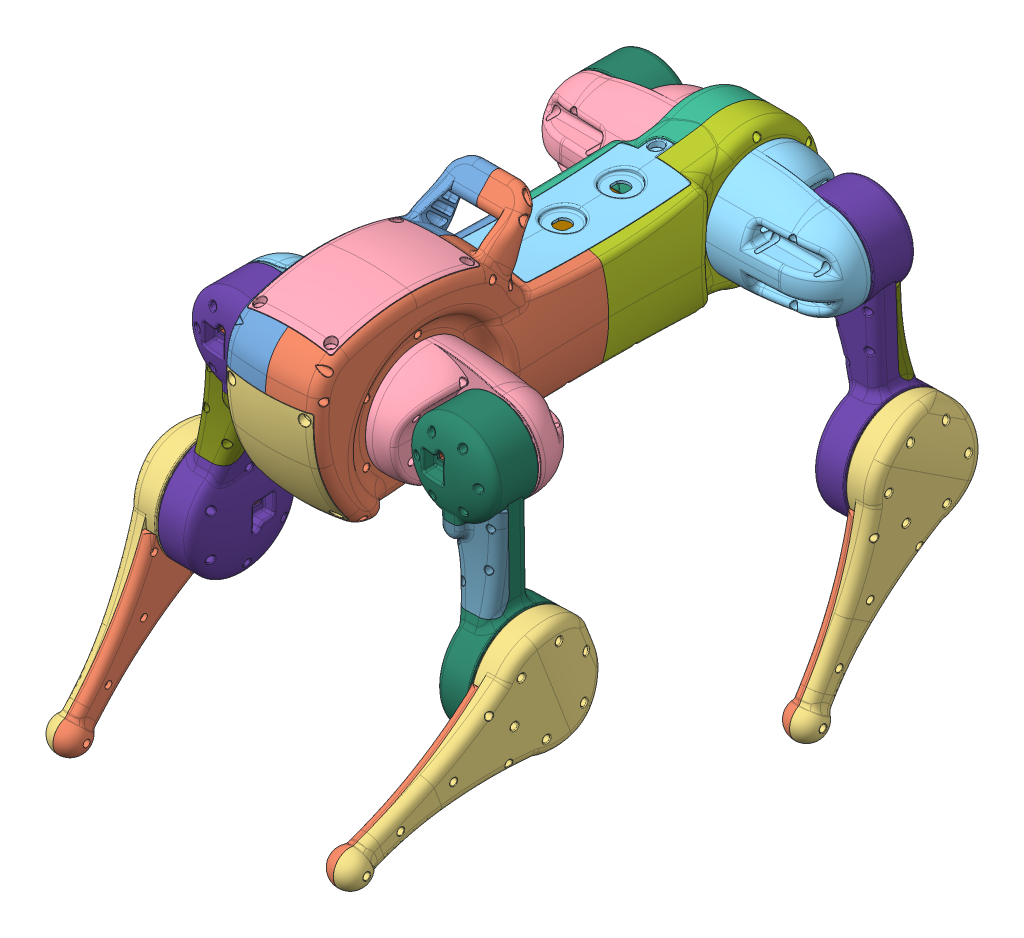
SolidWorks assembly ROBOT DOG, configuration Default. Lengths in mm.
Overall size (409.03 517.61 692.63).
101 component instances, 23 part files, 143 mates.
Components (placement in the parent):
- RIGHT FRONT TORSO - ROBOT DOG-1: RIGHT FRONT TORSO - ROBOT DOG [Default] at origin size (84.53 210.28 299.93)
- MirrorLEFT FRONT TORSO - ROBOT DOG-3: MirrorLEFT FRONT TORSO - ROBOT DOG [Default] x (-1 0 0) z (0 0 -1) size (91.07 210.28 299.93)
- COVER OF THE CAMERA BOARD - ROBOT DOG-1: COVER OF THE CAMERA BOARD - ROBOT DOG [Default] at origin size (89.79 121.01 49.11)
- COVER OF THE COMPUTER BOARD - ROBOT DOG-1: COVER OF THE COMPUTER BOARD - ROBOT DOG [Default] at origin size (87.15 28.45 157.74)
- COVER OF THE BATTERY - ROBOT DOG-1: COVER OF THE BATTERY - ROBOT DOG [Default] at origin size (83.94 31.1 211.37)
- RIGHT BACK TORSO - ROBOT DOG-2: RIGHT BACK TORSO - ROBOT DOG [Default] at origin size (84.66 140 246.51)
- MirrorLEFT BACK TORSO - ROBOT DOG-6: MirrorLEFT BACK TORSO - ROBOT DOG [Default] x (-1 0 0) z (0 0 -1) size (91.16 140 246.51)
- CONTROLLER BEHIND OF THE BATTERY - ROBOT DOG 38MM WITDH-1: CONTROLLER BEHIND OF THE BATTERY - ROBOT DOG 38MM WITDH [Default] at (0 -15.25 0) x (1 0 0) z (0 1 0) size (50 140 21.9)
- BATTERY - ROBOT DOG-1: BATTERY - ROBOT DOG [Default] at (0 8.05 -7) x (1 0 0) z (0 1 0) size (69 169 39)
- BIG PART - MOTOR 6-1: BIG PART - MOTOR 6 [Default] at (-113 -0.0192 -188.18) x (0 0.001455 0.999999) z (0.048855 0.998805 -0.001453) size (39.01 74 74)
  - PART 2 - MOTOR 6 - ROBOT DOG-1: PART 2 - MOTOR 6 - ROBOT DOG [Default] at origin size (33.16 74 74)
  - BIGGER CONTROLLER - ROBOT DOG-1: BIGGER CONTROLLER - ROBOT DOG [Default] at (-15.88 0 0) x (0 -1 0) z (0 0 -1) size (45 7.4 45)
- BIG PART - MOTOR 6-2: BIG PART - MOTOR 6 [Default] at (-113 0.0018 188.18) x (0 -0.000135 -1) z (0.008141 0.999967 -0.000135) size (39.01 74 74)
  - PART 2 - MOTOR 6 - ROBOT DOG-1: PART 2 - MOTOR 6 - ROBOT DOG [Default] at origin size (33.16 74 74)
  - BIGGER CONTROLLER - ROBOT DOG-1: BIGGER CONTROLLER - ROBOT DOG [Default] at (-15.88 0 0) x (0 -1 0) z (0 0 -1) size (45 7.4 45)
- BIG PART - MOTOR 6-3: BIG PART - MOTOR 6 [Default] at (113 0.1463 -188.1792) x (0 -0.011103 0.999938) z (-0.026827 0.999578 0.011099) size (39.01 74 74)
  - PART 2 - MOTOR 6 - ROBOT DOG-1: PART 2 - MOTOR 6 - ROBOT DOG [Default] at origin size (33.16 74 74)
  - BIGGER CONTROLLER - ROBOT DOG-1: BIGGER CONTROLLER - ROBOT DOG [Default] at (-15.88 0 0) x (0 -1 0) z (0 0 -1) size (45 7.4 45)
- BIG PART - MOTOR 6-4: BIG PART - MOTOR 6 [Default] at (113 0.1616 188.179) x (0 -0.012263 -0.999925) z (-0.027212 0.999555 -0.012259) size (39.01 74 74)
  - PART 2 - MOTOR 6 - ROBOT DOG-1: PART 2 - MOTOR 6 - ROBOT DOG [Default] at origin size (33.16 74 74)
  - BIGGER CONTROLLER - ROBOT DOG-1: BIGGER CONTROLLER - ROBOT DOG [Default] at (-15.88 0 0) x (0 -1 0) z (0 0 -1) size (45 7.4 45)
- SMALL PART - MOTOR 6-1: SMALL PART - MOTOR 6 [Default] at (113 -0.0619 169.9504) x (0 -0.012263 -0.999925) z (0.5 -0.86596 0.01062) size (5.8 74 74)
  - PART 1 - MOTOR 6 - ROBOT DOG-2: PART 1 - MOTOR 6 - ROBOT DOG [Default] at origin size (4.8 74 74)
  - SMALL CONTROLLER - ROBOT DOG-1: SMALL CONTROLLER - ROBOT DOG [Default] at (1.9 0 0) x (1 0 0) z (0 -0.5 0.866025) size (1 40.5 45)
- SMALL PART - MOTOR 6-2: SMALL PART - MOTOR 6 [Default] at (113 -0.0561 -169.9503) x (0 -0.011103 0.999938) z (0.5 0.865972 0.009616) size (5.8 74 74)
  - PART 1 - MOTOR 6 - ROBOT DOG-2: PART 1 - MOTOR 6 - ROBOT DOG [Default] at origin size (4.8 74 74)
  - SMALL CONTROLLER - ROBOT DOG-1: SMALL CONTROLLER - ROBOT DOG [Default] at (1.9 0 0) x (1 0 0) z (0 -0.5 0.866025) size (1 40.5 45)
- SMALL PART - MOTOR 6-3: SMALL PART - MOTOR 6 [Default] at (-113 0.0073 -169.95) x (0 0.001455 0.999999) z (-0.5 -0.866024 0.00126) size (5.8 74 74)
  - PART 1 - MOTOR 6 - ROBOT DOG-2: PART 1 - MOTOR 6 - ROBOT DOG [Default] at origin size (4.8 74 74)
  - SMALL CONTROLLER - ROBOT DOG-1: SMALL CONTROLLER - ROBOT DOG [Default] at (1.9 0 0) x (1 0 0) z (0 -0.5 0.866025) size (1 40.5 45)
- SMALL PART - MOTOR 6-4: SMALL PART - MOTOR 6 [Default] at (-113 -0.0007 169.95) x (0 -0.000135 -1) z (-0.5 0.866025 -0.000117) size (5.8 74 74)
  - PART 1 - MOTOR 6 - ROBOT DOG-2: PART 1 - MOTOR 6 - ROBOT DOG [Default] at origin size (4.8 74 74)
  - SMALL CONTROLLER - ROBOT DOG-1: SMALL CONTROLLER - ROBOT DOG [Default] at (1.9 0 0) x (1 0 0) z (0 -0.5 0.866025) size (1 40.5 45)
- COVER OF THE THIGN - ROBOT DOG-1: COVER OF THE THIGN - ROBOT DOG [Default] at (113 0.2046 191.6787) x (0.99963 0.02721 -0.000334) z (0 0.012263 0.999925) size (62.68 88.46 26.31)
- COVER OF THE THIGN - ROBOT DOG-2: COVER OF THE THIGN - ROBOT DOG [Default] at (-113 -0.0243 -191.68) x (-0.998806 0.048855 -0.000071) z (0 -0.001455 -0.999999) size (62.68 88.46 26.31)
- THIGN - ROBOT DOG-1: THIGN - ROBOT DOG [Default] at (-113 -0.0243 -191.68) x (-0.998806 0.048855 -0.000071) z (0 -0.001455 -0.999999) size (90.79 271.35 112.7)
- THIGN - ROBOT DOG-2: THIGN - ROBOT DOG [Default] at (113 0.2046 191.6787) x (0.99963 0.02721 -0.000334) z (0 0.012263 0.999925) size (90.79 271.35 112.7)
- MirrorCOVER OF THE THIGN - ROBOT DOG-4: MirrorCOVER OF THE THIGN - ROBOT DOG [Default] at (-113 0.0022 191.68) x (-0.999967 0.008141 -0.000001) z (0 -0.000135 -1) size (62.68 88.46 26.31)
- MirrorCOVER OF THE THIGN - ROBOT DOG-5: MirrorCOVER OF THE THIGN - ROBOT DOG [Default] at (113 0.1852 -191.679) x (0.99964 0.026825 0.000298) z (0 -0.011103 0.999938) size (62.68 88.46 26.31)
- MirrorANOTHER THIGN - ROBOT DOG-3: MirrorANOTHER THIGN - ROBOT DOG [Default] at (113 0.1852 -191.679) x (0.99964 0.026825 0.000298) z (0 -0.011103 0.999938) size (90.79 271.35 112.7)
- MirrorANOTHER THIGN - ROBOT DOG-4: MirrorANOTHER THIGN - ROBOT DOG [Default] at (-113 0.0022 191.68) x (-0.999967 0.008141 -0.000001) z (0 -0.000135 -1) size (90.79 271.35 112.7)
- BIG PART MOTOR 8-1: BIG PART MOTOR 8 [Default] at (24.425 0 175) size (30.55 96.7 96.7)
  - PART 2 - MOTOR 8 - ROBOT DOG-1: PART 2 - MOTOR 8 - ROBOT DOG [Default] at origin size (24.65 96.7 96.7)
  - BIGGER CONTROLLER - ROBOT DOG-1: BIGGER CONTROLLER - ROBOT DOG [Default] at (-11.675 0 0) x (0 0 1) z (0 -1 0) size (45 7.4 45)
- SMALL PART MOTOR 8-1: SMALL PART MOTOR 8 [Default] at (39.725 0 175) x (1 0 0) z (0 -0.859829 0.510583) size (8.45 96.7 96.7)
  - PART 1 - MOTOR 8 - ROBOT DOG-1: PART 1 - MOTOR 8 - ROBOT DOG [Default] at origin size (7.45 96.7 96.7)
  - SMALL CONTROLLER - ROBOT DOG-1: SMALL CONTROLLER - ROBOT DOG [Default] at (3.225 0 0) x (1 0 0) z (0 -0.5 0.866025) size (1 40.5 45)
- BIG PART MOTOR 8-2: BIG PART MOTOR 8 [Default] at (24.425 0 -175) size (30.55 96.7 96.7)
  - PART 2 - MOTOR 8 - ROBOT DOG-1: PART 2 - MOTOR 8 - ROBOT DOG [Default] at origin size (24.65 96.7 96.7)
  - BIGGER CONTROLLER - ROBOT DOG-1: BIGGER CONTROLLER - ROBOT DOG [Default] at (-11.675 0 0) x (0 0 1) z (0 -1 0) size (45 7.4 45)
- BIG PART MOTOR 8-3: BIG PART MOTOR 8 [Default] at (-24.425 0 175) x (-1 0 0) z (0 0 -1) size (30.55 96.7 96.7)
  - PART 2 - MOTOR 8 - ROBOT DOG-1: PART 2 - MOTOR 8 - ROBOT DOG [Default] at origin size (24.65 96.7 96.7)
  - BIGGER CONTROLLER - ROBOT DOG-1: BIGGER CONTROLLER - ROBOT DOG [Default] at (-11.675 0 0) x (0 0 1) z (0 -1 0) size (45 7.4 45)
- BIG PART MOTOR 8-4: BIG PART MOTOR 8 [Default] at (-24.425 0 -175) x (-1 0 0) z (0 0 -1) size (30.55 96.7 96.7)
  - PART 2 - MOTOR 8 - ROBOT DOG-1: PART 2 - MOTOR 8 - ROBOT DOG [Default] at origin size (24.65 96.7 96.7)
  - BIGGER CONTROLLER - ROBOT DOG-1: BIGGER CONTROLLER - ROBOT DOG [Default] at (-11.675 0 0) x (0 0 1) z (0 -1 0) size (45 7.4 45)
- SMALL PART MOTOR 8-2: SMALL PART MOTOR 8 [Default] at (39.725 0 -175) x (1 0 0) z (0 0.871524 -0.490354) size (8.45 96.7 96.7)
  - PART 1 - MOTOR 8 - ROBOT DOG-1: PART 1 - MOTOR 8 - ROBOT DOG [Default] at origin size (7.45 96.7 96.7)
  - SMALL CONTROLLER - ROBOT DOG-1: SMALL CONTROLLER - ROBOT DOG [Default] at (3.225 0 0) x (1 0 0) z (0 -0.5 0.866025) size (1 40.5 45)
- SMALL PART MOTOR 8-3: SMALL PART MOTOR 8 [Default] at (-39.725 0 175) x (-1 0 0) z (0 0.866093 0.499883) size (8.45 96.7 96.7)
  - PART 1 - MOTOR 8 - ROBOT DOG-1: PART 1 - MOTOR 8 - ROBOT DOG [Default] at origin size (7.45 96.7 96.7)
  - SMALL CONTROLLER - ROBOT DOG-1: SMALL CONTROLLER - ROBOT DOG [Default] at (3.225 0 0) x (1 0 0) z (0 -0.5 0.866025) size (1 40.5 45)
- SMALL PART MOTOR 8-4: SMALL PART MOTOR 8 [Default] at (-39.725 0 -175) x (-1 0 0) z (0 -0.866752 -0.49874) size (8.45 96.7 96.7)
  - PART 1 - MOTOR 8 - ROBOT DOG-1: PART 1 - MOTOR 8 - ROBOT DOG [Default] at origin size (7.45 96.7 96.7)
  - SMALL CONTROLLER - ROBOT DOG-1: SMALL CONTROLLER - ROBOT DOG [Default] at (3.225 0 0) x (1 0 0) z (0 -0.5 0.866025) size (1 40.5 45)
- BIG PART MOTOR 8-5: BIG PART MOTOR 8 [Default] at (150.9736 -168.8465 -193.5559) x (0.99964 0.026825 0.000298) z (0 0.011103 -0.999938) size (30.55 96.7 96.7)
  - PART 2 - MOTOR 8 - ROBOT DOG-1: PART 2 - MOTOR 8 - ROBOT DOG [Default] at origin size (24.65 96.7 96.7)
  - BIGGER CONTROLLER - ROBOT DOG-1: BIGGER CONTROLLER - ROBOT DOG [Default] at (-11.675 0 0) x (0 0 1) z (0 -1 0) size (45 7.4 45)
- BIG PART MOTOR 8-6: BIG PART MOTOR 8 [Default] at (151.0387 -168.8102 193.7516) x (0.99963 0.02721 -0.000334) z (0 -0.012263 -0.999925) size (30.55 96.7 96.7)
  - PART 2 - MOTOR 8 - ROBOT DOG-1: PART 2 - MOTOR 8 - ROBOT DOG [Default] at origin size (24.65 96.7 96.7)
  - BIGGER CONTROLLER - ROBOT DOG-1: BIGGER CONTROLLER - ROBOT DOG [Default] at (-11.675 0 0) x (0 0 1) z (0 -1 0) size (45 7.4 45)
- BIG PART MOTOR 8-7: BIG PART MOTOR 8 [Default] at (-154.6904 -168.1881 -191.4353) x (-0.998806 0.048855 -0.000071) z (0 0.001455 0.999999) size (30.55 96.7 96.7)
  - PART 2 - MOTOR 8 - ROBOT DOG-1: PART 2 - MOTOR 8 - ROBOT DOG [Default] at origin size (24.65 96.7 96.7)
  - BIGGER CONTROLLER - ROBOT DOG-1: BIGGER CONTROLLER - ROBOT DOG [Default] at (-11.675 0 0) x (0 0 1) z (0 -1 0) size (45 7.4 45)
- BIG PART MOTOR 8-8: BIG PART MOTOR 8 [Default] at (-147.8078 -169.72 191.7028) x (-0.999967 0.008141 -0.000001) z (0 0.000135 1) size (30.55 96.7 96.7)
  - PART 2 - MOTOR 8 - ROBOT DOG-1: PART 2 - MOTOR 8 - ROBOT DOG [Default] at origin size (24.65 96.7 96.7)
  - BIGGER CONTROLLER - ROBOT DOG-1: BIGGER CONTROLLER - ROBOT DOG [Default] at (-11.675 0 0) x (0 0 1) z (0 -1 0) size (45 7.4 45)
- SMALL PART MOTOR 8-5: SMALL PART MOTOR 8 [Default] at (166.2681 -168.4361 -193.5513) x (0.99964 0.026825 0.000298) z (-0.026771 0.998201 -0.05365) size (8.45 96.7 96.7)
  - PART 1 - MOTOR 8 - ROBOT DOG-1: PART 1 - MOTOR 8 - ROBOT DOG [Default] at origin size (7.45 96.7 96.7)
  - SMALL CONTROLLER - ROBOT DOG-1: SMALL CONTROLLER - ROBOT DOG [Default] at (3.225 0 0) x (1 0 0) z (0 -0.5 0.866025) size (1 40.5 45)
- SMALL PART MOTOR 8-6: SMALL PART MOTOR 8 [Default] at (166.3331 -168.3939 193.7465) x (0.99963 0.02721 -0.000334) z (-0.025425 0.938287 0.344921) size (8.45 96.7 96.7)
  - PART 1 - MOTOR 8 - ROBOT DOG-1: PART 1 - MOTOR 8 - ROBOT DOG [Default] at origin size (7.45 96.7 96.7)
  - SMALL CONTROLLER - ROBOT DOG-1: SMALL CONTROLLER - ROBOT DOG [Default] at (3.225 0 0) x (1 0 0) z (0 -0.5 0.866025) size (1 40.5 45)
- SMALL PART MOTOR 8-7: SMALL PART MOTOR 8 [Default] at (-169.9721 -167.4406 -191.4364) x (-0.998806 0.048855 -0.000071) z (-0.013599 -0.279414 -0.960074) size (8.45 96.7 96.7)
  - PART 1 - MOTOR 8 - ROBOT DOG-1: PART 1 - MOTOR 8 - ROBOT DOG [Default] at origin size (7.45 96.7 96.7)
  - SMALL CONTROLLER - ROBOT DOG-1: SMALL CONTROLLER - ROBOT DOG [Default] at (3.225 0 0) x (1 0 0) z (0 -0.5 0.866025) size (1 40.5 45)
- SMALL PART MOTOR 8-8: SMALL PART MOTOR 8 [Default] at (-163.1073 -169.5955 191.7028) x (-0.999967 0.008141 -0.000001) z (-0.00269 -0.330238 0.943894) size (8.45 96.7 96.7)
  - PART 1 - MOTOR 8 - ROBOT DOG-1: PART 1 - MOTOR 8 - ROBOT DOG [Default] at origin size (7.45 96.7 96.7)
  - SMALL CONTROLLER - ROBOT DOG-1: SMALL CONTROLLER - ROBOT DOG [Default] at (3.225 0 0) x (1 0 0) z (0 -0.5 0.866025) size (1 40.5 45)
- COVER OF THE LEG - ROBOT DOG-1: COVER OF THE LEG - ROBOT DOG [Default] at (164.6087 -168.4408 193.747) x (-0.99963 -0.02721 0.000334) z (0.025425 -0.938287 -0.344921) size (18.15 177.43 78.27)
- COVER OF THE LEG - ROBOT DOG-2: COVER OF THE LEG - ROBOT DOG [Default] at (164.5437 -168.4823 -193.5518) x (-0.99964 -0.026825 -0.000298) z (0.014889 -0.545539 -0.837953) size (18.15 177.43 78.27)
- COVER OF THE LEG - ROBOT DOG-3: COVER OF THE LEG - ROBOT DOG [Default] at (-161.3824 -169.6095 191.7028) x (0.999967 -0.008141 0.000001) z (0.00531 0.65229 0.757951) size (18.15 177.43 78.27)
- COVER OF THE LEG - ROBOT DOG-4: COVER OF THE LEG - ROBOT DOG [Default] at (-168.2492 -167.5249 -191.4363) x (0.998806 -0.048855 0.000071) z (0.047437 0.970162 0.237771) size (18.15 177.43 78.27)
- LEG - ROBOT DOG-1: LEG - ROBOT DOG [Default] at (-168.2492 -167.5249 -191.4363) x (0.998806 -0.048855 0.000071) z (0.047437 0.970162 0.237771) size (32.62 277.86 112.7)
- LEG - ROBOT DOG-2: LEG - ROBOT DOG [Default] at (-161.3824 -169.6095 191.7028) x (0.999967 -0.008141 0.000001) z (0.00531 0.65229 0.757951) size (32.62 277.86 112.7)
- LEG - ROBOT DOG-3: LEG - ROBOT DOG [Default] at (164.6087 -168.4408 193.747) x (-0.99963 -0.02721 0.000334) z (0.025425 -0.938287 -0.344921) size (32.62 277.86 112.7)
- LEG - ROBOT DOG-4: LEG - ROBOT DOG [Default] at (164.5437 -168.4823 -193.5518) x (-0.99964 -0.026825 -0.000298) z (0.014889 -0.545539 -0.837953) size (32.62 277.86 112.7)
- SHOULDER-1: SHOULDER [Default] at (38 0 175) x (1 0 0) z (0 0.012263 0.999925) size (122.68 117.46 115.67)
- SHOULDER-2: SHOULDER [Default] at (-38 0 -175) x (-1 0 0) z (0 -0.001455 -0.999999) size (122.68 117.46 115.67)
- MirrorSHOULDER-4: MirrorSHOULDER [Default] at (-38 0 175) x (-1 0 0) z (0 -0.000135 -1) size (122.68 117.46 115.67)
- MirrorSHOULDER-5: MirrorSHOULDER [Default] at (38 0 -175) x (1 0 0) z (0 -0.011103 0.999938) size (122.68 117.46 115.67)
Mates (geometry in assembly coordinates):
- Coincident1: coincident aligned: plane of RIGHT FRONT TORSO - ROBOT DOG-1 through (0 0 0) normal (0 0 1); plane of assembly through (0 0 0) normal (0 0 1)
- Coincident2: coincident aligned: plane of RIGHT FRONT TORSO - ROBOT DOG-1 through (0 0 0) normal (0 1 0); plane of assembly through (0 0 0) normal (0 1 0)
- Coincident3: coincident aligned: plane of RIGHT FRONT TORSO - ROBOT DOG-1 through (0 0 0) normal (1 0 0); plane of assembly through (0 0 0) normal (1 0 0)
- Concentric1: concentric anti-aligned: cylinder of RIGHT FRONT TORSO - ROBOT DOG-1 through (-8.35 0 175) axis (-1 0 0) radius 51.35; cylinder of MirrorLEFT FRONT TORSO - ROBOT DOG-3 through (8.35 0 175) axis (1 0 0) radius 51.35
- Coincident4: coincident aligned: plane of RIGHT FRONT TORSO - ROBOT DOG-1 through (0 0 0) normal (0 0 -1); plane of MirrorLEFT FRONT TORSO - ROBOT DOG-3 through (0 0 0) normal (0 0 -1)
- Coincident5: coincident anti-aligned: plane of RIGHT FRONT TORSO - ROBOT DOG-1 through (0 0 0) normal (1 0 0); plane of MirrorLEFT FRONT TORSO - ROBOT DOG-3 through (0 0 0) normal (-1 0 0)
- Concentric2: concentric aligned: cylinder of RIGHT FRONT TORSO - ROBOT DOG-1 through (-36.5 70.8966 265) axis (0 1 0) radius 2.865; cylinder of COVER OF THE COMPUTER BOARD - ROBOT DOG-1 through (-36.5 95 265) axis (0 1 0) radius 2.25
- Concentric3: concentric anti-aligned: cylinder of MirrorLEFT FRONT TORSO - ROBOT DOG-3 through (36.5 70.8966 125) axis (0 1 0) radius 2.865; cylinder of COVER OF THE COMPUTER BOARD - ROBOT DOG-1 through (36.5 117.4506 125) axis (0 -1 0) radius 5
- Coincident6: coincident anti-aligned: plane of MirrorLEFT FRONT TORSO - ROBOT DOG-3 through (500000 89 117.5) normal (0 1 0); plane of COVER OF THE COMPUTER BOARD - ROBOT DOG-1 through (0 89 0) normal (0 -1 0)
- Concentric4: concentric anti-aligned: cylinder of RIGHT FRONT TORSO - ROBOT DOG-1 through (-37.5 53.5018 266.4321) axis (0 -0.309017 0.951057) radius 2.865; cylinder of COVER OF THE CAMERA BOARD - ROBOT DOG-1 through (-37.5 32.6959 330.466) axis (0 0.309017 -0.951057) radius 5
- Concentric5: concentric anti-aligned: cylinder of MirrorLEFT FRONT TORSO - ROBOT DOG-3 through (37.5 -46.3592 233.9853) axis (0 -0.309017 0.951057) radius 2.865; cylinder of COVER OF THE CAMERA BOARD - ROBOT DOG-1 through (37.5 -67.1651 298.0192) axis (0 0.309017 -0.951057) radius 5
- Coincident7: coincident anti-aligned: plane of MirrorLEFT FRONT TORSO - ROBOT DOG-3 through (500000 -59.0864 248.8851) normal (0 -0.309017 0.951057); plane of COVER OF THE CAMERA BOARD - ROBOT DOG-1 through (0 -78.7877 242.4837) normal (0 0.309017 -0.951057)
- Concentric6: concentric anti-aligned: cylinder of MirrorLEFT FRONT TORSO - ROBOT DOG-3 through (10 0 75) axis (0 -1 0) radius 10; cylinder of COVER OF THE BATTERY - ROBOT DOG-1 through (10 37.6786 75) axis (0 1 0) radius 9.5
- Concentric7: concentric anti-aligned: cylinder of MirrorLEFT FRONT TORSO - ROBOT DOG-3 through (34 0 62) axis (0 -1 0) radius 3; cylinder of COVER OF THE BATTERY - ROBOT DOG-1 through (34 37.6786 62) axis (0 1 0) radius 2.5
- Coincident8: coincident anti-aligned: plane of MirrorLEFT FRONT TORSO - ROBOT DOG-3 through (20 50 65) normal (0 1 0); plane of COVER OF THE BATTERY - ROBOT DOG-1 through (0 50 0) normal (0 -1 0)
- Concentric8: concentric anti-aligned: cylinder of RIGHT FRONT TORSO - ROBOT DOG-1 through (-43.899 37.3651 1) axis (0 0 -1) radius 4; cylinder of RIGHT BACK TORSO - ROBOT DOG-2 through (-43.899 37.3651 3) axis (0 0 1) radius 1.7
- Concentric9: concentric anti-aligned: cylinder of RIGHT FRONT TORSO - ROBOT DOG-1 through (-8 -46.2757 1) axis (0 0 -1) radius 4; cylinder of RIGHT BACK TORSO - ROBOT DOG-2 through (-8 -46.2757 3) axis (0 0 1) radius 1.7
- Coincident9: coincident anti-aligned: plane of RIGHT FRONT TORSO - ROBOT DOG-1 through (0 0 0) normal (0 0 -1); plane of RIGHT BACK TORSO - ROBOT DOG-2 through (0 0 0) normal (0 0 1)
- Concentric10: concentric aligned: cylinder of MirrorLEFT FRONT TORSO - ROBOT DOG-3 through (43.899 37.3651 1) axis (0 0 -1) radius 4; cylinder of MirrorLEFT BACK TORSO - ROBOT DOG-6 through (43.899 37.3651 1) axis (0 0 -1) radius 3.75
- Concentric11: concentric aligned: cylinder of MirrorLEFT FRONT TORSO - ROBOT DOG-3 through (8 -46.2757 1) axis (0 0 -1) radius 4; cylinder of MirrorLEFT BACK TORSO - ROBOT DOG-6 through (8 -46.2757 1) axis (0 0 -1) radius 3.75
- Coincident10: coincident anti-aligned: plane of MirrorLEFT FRONT TORSO - ROBOT DOG-3 through (0 0 0) normal (0 0 -1); plane of MirrorLEFT BACK TORSO - ROBOT DOG-6 through (0 0 0) normal (0 0 1)
- Concentric12: concentric anti-aligned: cylinder of MirrorLEFT BACK TORSO - ROBOT DOG-6 through (19 -11.45 -66.5) axis (0 1 0) radius 1.7; cylinder of CONTROLLER BEHIND OF THE BATTERY - ROBOT DOG 38MM WITDH-1 through (19 -9.6003 -66.5) axis (0 -1 0) radius 1.75
- Concentric13: concentric anti-aligned: cylinder of MirrorLEFT BACK TORSO - ROBOT DOG-6 through (-19 -11.45 -66.5) axis (0 1 0) radius 1.7; cylinder of CONTROLLER BEHIND OF THE BATTERY - ROBOT DOG 38MM WITDH-1 through (-19 -9.6003 -66.5) axis (0 -1 0) radius 1.75
- Coincident11: coincident anti-aligned: plane of MirrorLEFT FRONT TORSO - ROBOT DOG-3 through (500000 -14.55 59) normal (0 -1 0); plane of CONTROLLER BEHIND OF THE BATTERY - ROBOT DOG 38MM WITDH-1 through (0 -14.55 0) normal (0 1 0)
- Coincident13: coincident aligned: plane of BATTERY - ROBOT DOG-1 through (0 8.05 -7) normal (1 0 0); plane of assembly through (0 0 0) normal (1 0 0)
- Width1: width anti-aligned: plane of RIGHT BACK TORSO - ROBOT DOG-2 through (-37 0 -107) normal (0 0 1); plane of MirrorLEFT FRONT TORSO - ROBOT DOG-3 through (500000 0 93) normal (0 0 -1); plane of BATTERY - ROBOT DOG-1 through (-34.5 27.55 -91.5) normal (0 0 -1); plane of BATTERY - ROBOT DOG-1 through (-34.5 27.55 77.5) normal (0 0 1)
- Coincident14: coincident anti-aligned: plane of MirrorLEFT FRONT TORSO - ROBOT DOG-3 through (500000 -11.45 59) normal (0 1 0); plane of BATTERY - ROBOT DOG-1 through (0 -11.45 -7) normal (0 -1 0)
- Coincident15: coincident anti-aligned: plane of BIG PART MOTOR 8-4/PART 2 - MOTOR 8 - ROBOT DOG-1 through (-35 0 -175) normal (-1 0 0); plane of SMALL PART MOTOR 8-4/PART 1 - MOTOR 8 - ROBOT DOG-1 through (-35 0 -175) normal (1 0 0)
- Concentric14: concentric aligned: cylinder of BIG PART MOTOR 8-4/PART 2 - MOTOR 8 - ROBOT DOG-1 through (-37 0 -175) axis (1 0 0) radius 48.35; cylinder of SMALL PART MOTOR 8-4/PART 1 - MOTOR 8 - ROBOT DOG-1 through (-42.45 0 -175) axis (1 0 0) radius 48.35
- Coincident16: coincident anti-aligned: plane of BIG PART MOTOR 8-3/PART 2 - MOTOR 8 - ROBOT DOG-1 through (-35 0 175) normal (-1 0 0); plane of SMALL PART MOTOR 8-3/PART 1 - MOTOR 8 - ROBOT DOG-1 through (-35 0 175) normal (1 0 0)
- Concentric15: concentric aligned: cylinder of BIG PART MOTOR 8-3/PART 2 - MOTOR 8 - ROBOT DOG-1 through (-37 0 175) axis (1 0 0) radius 48.35; cylinder of SMALL PART MOTOR 8-3/PART 1 - MOTOR 8 - ROBOT DOG-1 through (-42.45 0 175) axis (1 0 0) radius 48.35
- Coincident17: coincident anti-aligned: plane of BIG PART MOTOR 8-1/PART 2 - MOTOR 8 - ROBOT DOG-1 through (35 0 175) normal (1 0 0); plane of SMALL PART MOTOR 8-1/PART 1 - MOTOR 8 - ROBOT DOG-1 through (35 0 175) normal (-1 0 0)
- Concentric16: concentric aligned: cylinder of BIG PART MOTOR 8-1/PART 2 - MOTOR 8 - ROBOT DOG-1 through (37 0 175) axis (-1 0 0) radius 48.35; cylinder of SMALL PART MOTOR 8-1/PART 1 - MOTOR 8 - ROBOT DOG-1 through (42.45 0 175) axis (-1 0 0) radius 48.35
- Coincident18: coincident anti-aligned: plane of BIG PART MOTOR 8-2/PART 2 - MOTOR 8 - ROBOT DOG-1 through (35 0 -175) normal (1 0 0); plane of SMALL PART MOTOR 8-2/PART 1 - MOTOR 8 - ROBOT DOG-1 through (35 0 -175) normal (-1 0 0)
- Concentric17: concentric aligned: cylinder of BIG PART MOTOR 8-2/PART 2 - MOTOR 8 - ROBOT DOG-1 through (37 0 -175) axis (-1 0 0) radius 48.35; cylinder of SMALL PART MOTOR 8-2/PART 1 - MOTOR 8 - ROBOT DOG-1 through (42.45 0 -175) axis (-1 0 0) radius 48.35
- Concentric18: concentric aligned: cylinder of RIGHT BACK TORSO - ROBOT DOG-2 through (-6.85 43.35 -175) axis (1 0 0) radius 1.7; cylinder of BIG PART MOTOR 8-4/PART 2 - MOTOR 8 - ROBOT DOG-1 through (-14.85 43.35 -175) axis (1 0 0) radius 1.25
- Concentric19: concentric anti-aligned: cylinder of RIGHT BACK TORSO - ROBOT DOG-2 through (-8.35 0 -175) axis (-1 0 0) radius 48.85; cylinder of BIG PART MOTOR 8-4/PART 2 - MOTOR 8 - ROBOT DOG-1 through (-37 0 -175) axis (1 0 0) radius 48.35
- Coincident19: coincident anti-aligned: plane of RIGHT BACK TORSO - ROBOT DOG-2 through (-11.85 43.35 -175) normal (-1 0 0); plane of BIG PART MOTOR 8-4/PART 2 - MOTOR 8 - ROBOT DOG-1 through (-11.85 0 -175) normal (1 0 0)
- Concentric20: concentric aligned: cylinder of MirrorLEFT BACK TORSO - ROBOT DOG-6 through (6.85 43.35 -175) axis (-1 0 0) radius 1.7; cylinder of BIG PART MOTOR 8-2/PART 2 - MOTOR 8 - ROBOT DOG-1 through (14.85 43.35 -175) axis (-1 0 0) radius 1.25
- Concentric21: concentric anti-aligned: cylinder of MirrorLEFT BACK TORSO - ROBOT DOG-6 through (8.35 0 -175) axis (1 0 0) radius 48.85; cylinder of BIG PART MOTOR 8-2/PART 2 - MOTOR 8 - ROBOT DOG-1 through (37 0 -175) axis (-1 0 0) radius 48.35
- Coincident20: coincident anti-aligned: plane of MirrorLEFT BACK TORSO - ROBOT DOG-6 through (11.85 43.35 -175) normal (1 0 0); plane of BIG PART MOTOR 8-2/PART 2 - MOTOR 8 - ROBOT DOG-1 through (11.85 0 -175) normal (-1 0 0)
- Concentric22: concentric aligned: cylinder of RIGHT FRONT TORSO - ROBOT DOG-1 through (-6.85 43.35 175) axis (1 0 0) radius 1.7; cylinder of BIG PART MOTOR 8-3/PART 2 - MOTOR 8 - ROBOT DOG-1 through (-14.85 43.35 175) axis (1 0 0) radius 1.25
- Concentric23: concentric anti-aligned: cylinder of RIGHT FRONT TORSO - ROBOT DOG-1 through (-8.35 0 175) axis (-1 0 0) radius 48.85; cylinder of BIG PART MOTOR 8-3/PART 2 - MOTOR 8 - ROBOT DOG-1 through (-37 0 175) axis (1 0 0) radius 48.35
- Coincident21: coincident anti-aligned: plane of RIGHT FRONT TORSO - ROBOT DOG-1 through (-11.85 43.35 175) normal (-1 0 0); plane of BIG PART MOTOR 8-3/PART 2 - MOTOR 8 - ROBOT DOG-1 through (-11.85 0 175) normal (1 0 0)
- Concentric24: concentric aligned: cylinder of MirrorLEFT FRONT TORSO - ROBOT DOG-3 through (6.85 43.35 175) axis (-1 0 0) radius 1.7; cylinder of BIG PART MOTOR 8-1/PART 2 - MOTOR 8 - ROBOT DOG-1 through (14.85 43.35 175) axis (-1 0 0) radius 1.25
- Concentric25: concentric anti-aligned: cylinder of MirrorLEFT FRONT TORSO - ROBOT DOG-3 through (8.35 0 175) axis (1 0 0) radius 48.85; cylinder of BIG PART MOTOR 8-1/PART 2 - MOTOR 8 - ROBOT DOG-1 through (37 0 175) axis (-1 0 0) radius 48.35
- Coincident22: coincident anti-aligned: plane of MirrorLEFT FRONT TORSO - ROBOT DOG-3 through (11.85 43.35 175) normal (1 0 0); plane of BIG PART MOTOR 8-1/PART 2 - MOTOR 8 - ROBOT DOG-1 through (11.85 0 175) normal (-1 0 0)
- Coincident27: coincident anti-aligned: plane of BIG PART - MOTOR 6-4/PART 2 - MOTOR 6 - ROBOT DOG-1 through (113 -0.0202 173.3501) normal (0 -0.012263 -0.999925); plane of SMALL PART - MOTOR 6-1/PART 1 - MOTOR 6 - ROBOT DOG-2 through (113 -0.0202 173.3501) normal (0 0.012263 0.999925)
- Concentric34: concentric aligned: cylinder of BIG PART - MOTOR 6-4/PART 2 - MOTOR 6 - ROBOT DOG-1 through (113 -0.0448 171.3503) axis (0 0.012263 0.999925) radius 37; cylinder of SMALL PART - MOTOR 6-1/PART 1 - MOTOR 6 - ROBOT DOG-2 through (113 -0.0791 168.5505) axis (0 0.012263 0.999925) radius 37
- Coincident28: coincident anti-aligned: plane of BIG PART - MOTOR 6-3/PART 2 - MOTOR 6 - ROBOT DOG-1 through (113 -0.0183 -173.3501) normal (0 -0.011103 0.999938); plane of SMALL PART - MOTOR 6-2/PART 1 - MOTOR 6 - ROBOT DOG-2 through (113 -0.0183 -173.3501) normal (0 0.011103 -0.999938)
- Concentric35: concentric aligned: cylinder of BIG PART - MOTOR 6-3/PART 2 - MOTOR 6 - ROBOT DOG-1 through (113 -0.0405 -171.3502) axis (0 0.011103 -0.999938) radius 37; cylinder of SMALL PART - MOTOR 6-2/PART 1 - MOTOR 6 - ROBOT DOG-2 through (113 -0.0716 -168.5504) axis (0 0.011103 -0.999938) radius 37
- Coincident29: coincident anti-aligned: plane of BIG PART - MOTOR 6-1/PART 2 - MOTOR 6 - ROBOT DOG-1 through (-113 0.0024 -173.35) normal (0 0.001455 0.999999); plane of SMALL PART - MOTOR 6-3/PART 1 - MOTOR 6 - ROBOT DOG-2 through (-113 0.0024 -173.35) normal (0 -0.001455 -0.999999)
- Concentric36: concentric aligned: cylinder of BIG PART - MOTOR 6-1/PART 2 - MOTOR 6 - ROBOT DOG-1 through (-113 0.0053 -171.35) axis (0 -0.001455 -0.999999) radius 37; cylinder of SMALL PART - MOTOR 6-3/PART 1 - MOTOR 6 - ROBOT DOG-2 through (-113 0.0094 -168.55) axis (0 -0.001455 -0.999999) radius 37
- Coincident30: coincident anti-aligned: plane of BIG PART - MOTOR 6-2/PART 2 - MOTOR 6 - ROBOT DOG-1 through (-113 -0.0002 173.35) normal (0 -0.000135 -1); plane of SMALL PART - MOTOR 6-4/PART 1 - MOTOR 6 - ROBOT DOG-2 through (-113 -0.0002 173.35) normal (0 0.000135 1)
- Concentric37: concentric aligned: cylinder of BIG PART - MOTOR 6-2/PART 2 - MOTOR 6 - ROBOT DOG-1 through (-113 -0.0005 171.35) axis (0 0.000135 1) radius 37; cylinder of SMALL PART - MOTOR 6-4/PART 1 - MOTOR 6 - ROBOT DOG-2 through (-113 -0.0009 168.55) axis (0 0.000135 1) radius 37
- Concentric47: concentric aligned: cylinder of COVER OF THE THIGN - ROBOT DOG-1 through (113 0.8956 248.0255) axis (0 -0.012263 -0.999925) radius 45; cylinder of THIGN - ROBOT DOG-2 through (113 0.4416 211.0073) axis (0 -0.012263 -0.999925) radius 45
- Concentric48: concentric aligned: cylinder of COVER OF THE THIGN - ROBOT DOG-1 through (92.1995 -98.7628 215.5642) axis (0.99963 0.02721 -0.000334) radius 15; cylinder of THIGN - ROBOT DOG-2 through (70.7012 -99.348 215.5714) axis (0.99963 0.02721 -0.000334) radius 15
- Concentric49: concentric aligned: cylinder of COVER OF THE THIGN - ROBOT DOG-2 through (-113 -0.1062 -248.0309) axis (0 0.001455 0.999999) radius 45; cylinder of THIGN - ROBOT DOG-1 through (-113 -0.0524 -211.01) axis (0 0.001455 0.999999) radius 45
- Concentric50: concentric aligned: cylinder of COVER OF THE THIGN - ROBOT DOG-2 through (-94.3539 -99.7371 -214.2049) axis (-0.998806 0.048855 -0.000071) radius 15; cylinder of THIGN - ROBOT DOG-1 through (-72.8732 -100.7878 -214.2034) axis (-0.998806 0.048855 -0.000071) radius 15
- Concentric51: concentric anti-aligned: cylinder of BIG PART - MOTOR 6-4/PART 2 - MOTOR 6 - ROBOT DOG-1 through (96.5135 27.1249 197.9791) axis (0 0.012263 0.999925) radius 1.25; cylinder of THIGN - ROBOT DOG-2 through (96.5135 27.7347 247.6963) axis (0 -0.012263 -0.999925) radius 3.5
- Concentric52: concentric anti-aligned: cylinder of BIG PART - MOTOR 6-4/PART 2 - MOTOR 6 - ROBOT DOG-1 through (113 -0.0448 171.3503) axis (0 0.012263 0.999925) radius 37; cylinder of THIGN - ROBOT DOG-2 through (113 0.4416 211.0073) axis (0 -0.012263 -0.999925) radius 45
- Coincident35: coincident anti-aligned: plane of BIG PART - MOTOR 6-4/PART 2 - MOTOR 6 - ROBOT DOG-1 through (113 0.368 205.0077) normal (0 0.012263 0.999925); plane of THIGN - ROBOT DOG-2 through (81.5117 -0.4891 205.0183) normal (0 -0.012263 -0.999925)
- Concentric53: concentric anti-aligned: cylinder of BIG PART - MOTOR 6-1/PART 2 - MOTOR 6 - ROBOT DOG-1 through (-113 0.0053 -171.35) axis (0 -0.001455 -0.999999) radius 37; cylinder of THIGN - ROBOT DOG-1 through (-113 -0.0524 -211.01) axis (0 0.001455 0.999999) radius 45
- Concentric54: concentric anti-aligned: cylinder of THIGN - ROBOT DOG-1 through (-95.9361 26.3715 -248.0694) axis (0 0.001455 0.999999) radius 3.5; cylinder of BIG PART - MOTOR 6-1/PART 2 - MOTOR 6 - ROBOT DOG-1 through (-95.9361 26.4438 -198.3485) axis (0 -0.001455 -0.999999) radius 1.25
- Coincident36: coincident anti-aligned: plane of BIG PART - MOTOR 6-1/PART 2 - MOTOR 6 - ROBOT DOG-1 through (-113 -0.0437 -205.01) normal (0 -0.001455 -0.999999); plane of THIGN - ROBOT DOG-1 through (-81.5376 -1.5826 -205.0077) normal (0 0.001455 0.999999)
- Concentric55: concentric aligned: cylinder of MirrorCOVER OF THE THIGN - ROBOT DOG-5 through (113 0.8109 -248.0265) axis (0 -0.011103 0.999938) radius 45; cylinder of MirrorANOTHER THIGN - ROBOT DOG-3 through (113 0.3998 -211.0078) axis (0 -0.011103 0.999938) radius 45
- Concentric56: concentric aligned: cylinder of MirrorCOVER OF THE THIGN - ROBOT DOG-5 through (92.1613 -98.8017 -215.4495) axis (0.99964 0.026825 0.000298) radius 15; cylinder of MirrorANOTHER THIGN - ROBOT DOG-3 through (70.6627 -99.3786 -215.4559) axis (0.99964 0.026825 0.000298) radius 15
- Concentric57: concentric aligned: cylinder of MirrorCOVER OF THE THIGN - ROBOT DOG-4 through (-113 0.0098 248.031) axis (0 -0.000135 -1) radius 45; cylinder of MirrorANOTHER THIGN - ROBOT DOG-4 through (-113 0.0048 211.01) axis (0 -0.000135 -1) radius 45
- Concentric58: concentric aligned: cylinder of MirrorCOVER OF THE THIGN - ROBOT DOG-4 through (-90.3102 -98.8327 214.3633) axis (-0.999967 0.008141 -0.000001) radius 15; cylinder of MirrorANOTHER THIGN - ROBOT DOG-4 through (-68.8046 -99.0078 214.3633) axis (-0.999967 0.008141 -0.000001) radius 15
- Concentric61: concentric anti-aligned: cylinder of BIG PART - MOTOR 6-2/PART 2 - MOTOR 6 - ROBOT DOG-1 through (-128.5274 27.4103 198.3063) axis (0 0.000135 1) radius 1.25; cylinder of MirrorANOTHER THIGN - ROBOT DOG-4 through (-128.5274 27.4169 248.0273) axis (0 -0.000135 -1) radius 3.5
- Concentric62: concentric anti-aligned: cylinder of BIG PART - MOTOR 6-2/PART 2 - MOTOR 6 - ROBOT DOG-1 through (-113 -0.0005 171.35) axis (0 0.000135 1) radius 37; cylinder of MirrorANOTHER THIGN - ROBOT DOG-4 through (-113 0.0048 211.01) axis (0 -0.000135 -1) radius 45
- Coincident37: coincident anti-aligned: plane of BIG PART - MOTOR 6-2/PART 2 - MOTOR 6 - ROBOT DOG-1 through (-113 0.004 205.01) normal (0 0.000135 1); plane of MirrorANOTHER THIGN - ROBOT DOG-4 through (-81.501 -0.2524 205.01) normal (0 -0.000135 -1)
- Concentric63: concentric anti-aligned: cylinder of BIG PART - MOTOR 6-3/PART 2 - MOTOR 6 - ROBOT DOG-1 through (128.0125 27.9496 -198.0011) axis (0 0.011103 -0.999938) radius 1.25; cylinder of MirrorANOTHER THIGN - ROBOT DOG-3 through (128.0125 28.5017 -247.719) axis (0 -0.011103 0.999938) radius 3.5
- Concentric64: concentric anti-aligned: cylinder of BIG PART - MOTOR 6-3/PART 2 - MOTOR 6 - ROBOT DOG-1 through (113 -0.0405 -171.3502) axis (0 0.011103 -0.999938) radius 37; cylinder of MirrorANOTHER THIGN - ROBOT DOG-3 through (113 0.3998 -211.0078) axis (0 -0.011103 0.999938) radius 45
- Coincident38: coincident anti-aligned: plane of BIG PART - MOTOR 6-3/PART 2 - MOTOR 6 - ROBOT DOG-1 through (113 0.3332 -205.0082) normal (0 0.011103 -0.999938); plane of MirrorANOTHER THIGN - ROBOT DOG-3 through (81.5113 -0.5118 -205.0175) normal (0 -0.011103 0.999938)
- Coincident39: coincident anti-aligned: plane of BIG PART MOTOR 8-6/PART 2 - MOTOR 8 - ROBOT DOG-1 through (161.6098 -168.5225 193.748) normal (0.99963 0.02721 -0.000334); plane of SMALL PART MOTOR 8-6/PART 1 - MOTOR 8 - ROBOT DOG-1 through (161.6098 -168.5225 193.748) normal (-0.99963 -0.02721 0.000334)
- Concentric65: concentric aligned: cylinder of BIG PART MOTOR 8-6/PART 2 - MOTOR 8 - ROBOT DOG-1 through (163.6091 -168.468 193.7474) axis (-0.99963 -0.02721 0.000334) radius 48.35; cylinder of SMALL PART MOTOR 8-6/PART 1 - MOTOR 8 - ROBOT DOG-1 through (169.057 -168.3197 193.7456) axis (-0.99963 -0.02721 0.000334) radius 48.35
- Coincident40: coincident anti-aligned: plane of BIG PART MOTOR 8-5/PART 2 - MOTOR 8 - ROBOT DOG-1 through (161.5448 -168.5628 -193.5527) normal (0.99964 0.026825 0.000298); plane of SMALL PART MOTOR 8-5/PART 1 - MOTOR 8 - ROBOT DOG-1 through (161.5448 -168.5628 -193.5527) normal (-0.99964 -0.026825 -0.000298)
- Concentric66: concentric aligned: cylinder of BIG PART MOTOR 8-5/PART 2 - MOTOR 8 - ROBOT DOG-1 through (163.544 -168.5092 -193.5521) axis (-0.99964 -0.026825 -0.000298) radius 48.35; cylinder of SMALL PART MOTOR 8-5/PART 1 - MOTOR 8 - ROBOT DOG-1 through (168.9921 -168.363 -193.5505) axis (-0.99964 -0.026825 -0.000298) radius 48.35
- Coincident41: coincident anti-aligned: plane of BIG PART MOTOR 8-7/PART 2 - MOTOR 8 - ROBOT DOG-1 through (-165.2528 -167.6715 -191.4361) normal (-0.998806 0.048855 -0.000071); plane of SMALL PART MOTOR 8-7/PART 1 - MOTOR 8 - ROBOT DOG-1 through (-165.2528 -167.6715 -191.4361) normal (0.998806 -0.048855 0.000071)
- Concentric67: concentric aligned: cylinder of BIG PART MOTOR 8-7/PART 2 - MOTOR 8 - ROBOT DOG-1 through (-167.2504 -167.5738 -191.4362) axis (0.998806 -0.048855 0.000071) radius 48.35; cylinder of SMALL PART MOTOR 8-7/PART 1 - MOTOR 8 - ROBOT DOG-1 through (-172.6939 -167.3075 -191.4366) axis (0.998806 -0.048855 0.000071) radius 48.35
- Coincident42: coincident anti-aligned: plane of BIG PART MOTOR 8-8/PART 2 - MOTOR 8 - ROBOT DOG-1 through (-158.3825 -169.6339 191.7028) normal (-0.999967 0.008141 -0.000001); plane of SMALL PART MOTOR 8-8/PART 1 - MOTOR 8 - ROBOT DOG-1 through (-158.3825 -169.6339 191.7028) normal (0.999967 -0.008141 0.000001)
- Concentric68: concentric aligned: cylinder of BIG PART MOTOR 8-8/PART 2 - MOTOR 8 - ROBOT DOG-1 through (-160.3824 -169.6176 191.7028) axis (0.999967 -0.008141 0.000001) radius 48.35; cylinder of SMALL PART MOTOR 8-8/PART 1 - MOTOR 8 - ROBOT DOG-1 through (-165.8322 -169.5733 191.7028) axis (0.999967 -0.008141 0.000001) radius 48.35
- Concentric69: concentric anti-aligned: cylinder of MirrorANOTHER THIGN - ROBOT DOG-3 through (73.7397 -214.282 -194.0604) axis (0.99964 0.026825 0.000298) radius 3.5; cylinder of BIG PART MOTOR 8-5/PART 2 - MOTOR 8 - ROBOT DOG-1 through (142.565 -212.4351 -194.0399) axis (-0.99964 -0.026825 -0.000298) radius 1.25
- Concentric70: concentric anti-aligned: cylinder of MirrorANOTHER THIGN - ROBOT DOG-3 through (135.4042 -169.2643 -193.5605) axis (0.99964 0.026825 0.000298) radius 56.35; cylinder of BIG PART MOTOR 8-5/PART 2 - MOTOR 8 - ROBOT DOG-1 through (163.544 -168.5092 -193.5521) axis (-0.99964 -0.026825 -0.000298) radius 48.35
- Coincident43: coincident anti-aligned: plane of MirrorANOTHER THIGN - ROBOT DOG-3 through (139.566 -212.5156 -194.0408) normal (0.99964 0.026825 0.000298); plane of BIG PART MOTOR 8-5/PART 2 - MOTOR 8 - ROBOT DOG-1 through (138.4031 -169.1838 -193.5596) normal (-0.99964 -0.026825 -0.000298)
- Concentric71: concentric anti-aligned: cylinder of THIGN - ROBOT DOG-2 through (73.8224 -214.2749 194.3092) axis (0.99963 0.02721 -0.000334) radius 3.5; cylinder of BIG PART MOTOR 8-6/PART 2 - MOTOR 8 - ROBOT DOG-1 through (142.6469 -212.4014 194.2862) axis (-0.99963 -0.02721 0.000334) radius 1.25
- Concentric72: concentric anti-aligned: cylinder of THIGN - ROBOT DOG-2 through (135.4695 -169.234 193.7568) axis (0.99963 0.02721 -0.000334) radius 56.35; cylinder of BIG PART MOTOR 8-6/PART 2 - MOTOR 8 - ROBOT DOG-1 through (163.6091 -168.468 193.7474) axis (-0.99963 -0.02721 0.000334) radius 48.35
- Coincident44: coincident anti-aligned: plane of THIGN - ROBOT DOG-2 through (139.648 -212.4831 194.2872) normal (0.99963 0.02721 -0.000334); plane of BIG PART MOTOR 8-6/PART 2 - MOTOR 8 - ROBOT DOG-1 through (138.4684 -169.1524 193.7558) normal (-0.99963 -0.02721 0.000334)
- Concentric73: concentric anti-aligned: cylinder of THIGN - ROBOT DOG-1 through (-78.4769 -215.3177 -191.3668) axis (-0.998806 0.048855 -0.000071) radius 3.5; cylinder of BIG PART MOTOR 8-7/PART 2 - MOTOR 8 - ROBOT DOG-1 through (-147.2447 -211.9541 -191.3717) axis (0.998806 -0.048855 0.000071) radius 1.25
- Concentric74: concentric anti-aligned: cylinder of THIGN - ROBOT DOG-1 through (-139.134 -168.949 -191.4342) axis (-0.998806 0.048855 -0.000071) radius 56.35; cylinder of BIG PART MOTOR 8-7/PART 2 - MOTOR 8 - ROBOT DOG-1 through (-167.2504 -167.5738 -191.4362) axis (0.998806 -0.048855 0.000071) radius 48.35
- Coincident45: coincident anti-aligned: plane of THIGN - ROBOT DOG-1 through (-144.2482 -212.1007 -191.3714) normal (-0.998806 0.048855 -0.000071); plane of BIG PART MOTOR 8-7/PART 2 - MOTOR 8 - ROBOT DOG-1 through (-142.1304 -168.8025 -191.4344) normal (0.998806 -0.048855 0.000071)
- Concentric75: concentric anti-aligned: cylinder of MirrorANOTHER THIGN - ROBOT DOG-4 through (-69.7383 -213.707 191.7088) axis (-0.999967 0.008141 -0.000001) radius 3.5; cylinder of BIG PART MOTOR 8-8/PART 2 - MOTOR 8 - ROBOT DOG-1 through (-138.5861 -213.1465 191.7087) axis (0.999967 -0.008141 0.000001) radius 1.25
- Concentric76: concentric anti-aligned: cylinder of MirrorANOTHER THIGN - ROBOT DOG-4 through (-132.2334 -169.8468 191.7029) axis (-0.999967 0.008141 -0.000001) radius 56.35; cylinder of BIG PART MOTOR 8-8/PART 2 - MOTOR 8 - ROBOT DOG-1 through (-160.3824 -169.6176 191.7028) axis (0.999967 -0.008141 0.000001) radius 48.35
- Coincident46: coincident anti-aligned: plane of MirrorANOTHER THIGN - ROBOT DOG-4 through (-135.5862 -213.1709 191.7087) normal (-0.999967 0.008141 -0.000001); plane of BIG PART MOTOR 8-8/PART 2 - MOTOR 8 - ROBOT DOG-1 through (-135.2333 -169.8224 191.7029) normal (0.999967 -0.008141 0.000001)
- Concentric77: concentric anti-aligned: cylinder of COVER OF THE LEG - ROBOT DOG-4 through (-160.7581 -167.8913 -191.4358) axis (-0.998806 0.048855 -0.000071) radius 56.35; cylinder of LEG - ROBOT DOG-1 through (-198.4805 -166.0462 -191.4384) axis (0.998806 -0.048855 0.000071) radius 56.35
- Concentric78: concentric anti-aligned: cylinder of COVER OF THE LEG - ROBOT DOG-4 through (-163.1421 -216.3414 6.7272) axis (-0.998806 0.048855 -0.000071) radius 3.5; cylinder of LEG - ROBOT DOG-1 through (-208.9852 -214.099 6.724) axis (0.998806 -0.048855 0.000071) radius 3.5
- Coincident47: coincident anti-aligned: plane of COVER OF THE LEG - ROBOT DOG-4 through (-178.2372 -167.0364 -191.437) normal (-0.998806 0.048855 -0.000071); plane of LEG - ROBOT DOG-1 through (-178.2372 -167.0364 -191.437) normal (0.998806 -0.048855 0.000071)
- Concentric79: concentric anti-aligned: cylinder of COVER OF THE LEG - ROBOT DOG-3 through (-154.0858 -194.6204 248.8429) axis (-0.999967 0.008141 -0.000001) radius 3.5; cylinder of LEG - ROBOT DOG-2 through (-199.9822 -194.2467 248.8428) axis (0.999967 -0.008141 0.000001) radius 3.5
- Concentric80: concentric anti-aligned: cylinder of COVER OF THE LEG - ROBOT DOG-3 through (-155.1416 -324.2979 324.7835) axis (-0.999967 0.008141 -0.000001) radius 3.5; cylinder of LEG - ROBOT DOG-2 through (-201.038 -323.9242 324.7835) axis (0.999967 -0.008141 0.000001) radius 3.5
- Coincident48: coincident anti-aligned: plane of COVER OF THE LEG - ROBOT DOG-3 through (-171.3821 -169.5281 191.7028) normal (-0.999967 0.008141 -0.000001); plane of LEG - ROBOT DOG-2 through (-171.3821 -169.5281 191.7028) normal (0.999967 -0.008141 0.000001)
- Concentric81: concentric anti-aligned: cylinder of COVER OF THE LEG - ROBOT DOG-1 through (158.3437 -213.3819 237.1616) axis (0.99963 0.02721 -0.000334) radius 3.5; cylinder of LEG - ROBOT DOG-3 through (204.2247 -212.133 237.1463) axis (-0.99963 -0.02721 0.000334) radius 3.5
- Concentric82: concentric anti-aligned: cylinder of COVER OF THE LEG - ROBOT DOG-1 through (159.0901 -238.9858 385.2434) axis (0.99963 0.02721 -0.000334) radius 3.5; cylinder of LEG - ROBOT DOG-3 through (204.9711 -237.7369 385.2281) axis (-0.99963 -0.02721 0.000334) radius 3.5
- Coincident49: coincident anti-aligned: plane of COVER OF THE LEG - ROBOT DOG-1 through (174.605 -168.1687 193.7437) normal (0.99963 0.02721 -0.000334); plane of LEG - ROBOT DOG-3 through (174.605 -168.1687 193.7437) normal (-0.99963 -0.02721 0.000334)
- Concentric83: concentric anti-aligned: cylinder of COVER OF THE LEG - ROBOT DOG-2 through (161.5991 -339.577 -82.2151) axis (0.99964 0.026825 0.000298) radius 3.5; cylinder of LEG - ROBOT DOG-4 through (207.4805 -338.3458 -82.2014) axis (-0.99964 -0.026825 -0.000298) radius 3.5
- Coincident50: coincident anti-aligned: plane of COVER OF THE LEG - ROBOT DOG-2 through (174.5401 -168.2141 -193.5488) normal (0.99964 0.026825 0.000298); plane of LEG - ROBOT DOG-4 through (174.5401 -168.2141 -193.5488) normal (-0.99964 -0.026825 -0.000298)
- Concentric84: concentric anti-aligned: cylinder of SMALL PART MOTOR 8-8/PART 1 - MOTOR 8 - ROBOT DOG-1 through (-163.0823 -200.2937 218.1215) axis (-0.999967 0.008141 -0.000001) radius 1.25; cylinder of LEG - ROBOT DOG-2 through (-200.029 -199.9929 218.1214) axis (0.999967 -0.008141 0.000001) radius 3.5
- Concentric85: concentric aligned: cylinder of BIG PART MOTOR 8-8/PART 2 - MOTOR 8 - ROBOT DOG-1 through (-160.3824 -169.6176 191.7028) axis (0.999967 -0.008141 0.000001) radius 48.35; cylinder of LEG - ROBOT DOG-2 through (-191.6488 -169.3631 191.7028) axis (0.999967 -0.008141 0.000001) radius 56.35
- Coincident51: coincident anti-aligned: plane of SMALL PART MOTOR 8-8/PART 1 - MOTOR 8 - ROBOT DOG-1 through (-165.8322 -169.5733 191.7028) normal (-0.999967 0.008141 -0.000001); plane of LEG - ROBOT DOG-2 through (-165.5823 -138.8773 165.2842) normal (0.999967 -0.008141 0.000001)
- Concentric86: concentric anti-aligned: cylinder of SMALL PART MOTOR 8-7/PART 1 - MOTOR 8 - ROBOT DOG-1 through (-169.2242 -157.836 -230.7749) axis (-0.998806 0.048855 -0.000071) radius 1.25; cylinder of LEG - ROBOT DOG-1 through (-206.128 -156.0309 -230.7775) axis (0.998806 -0.048855 0.000071) radius 3.5
- Concentric87: concentric aligned: cylinder of SMALL PART MOTOR 8-7/PART 1 - MOTOR 8 - ROBOT DOG-1 through (-172.6939 -167.3075 -191.4366) axis (0.998806 -0.048855 0.000071) radius 48.35; cylinder of LEG - ROBOT DOG-1 through (-198.4805 -166.0462 -191.4384) axis (0.998806 -0.048855 0.000071) radius 56.35
- Coincident52: coincident anti-aligned: plane of SMALL PART MOTOR 8-7/PART 1 - MOTOR 8 - ROBOT DOG-1 through (-172.6939 -167.3075 -191.4366) normal (-0.998806 0.048855 -0.000071); plane of LEG - ROBOT DOG-1 through (-172.2206 -157.6894 -230.7751) normal (0.998806 -0.048855 0.000071)
- Concentric88: concentric aligned: cylinder of SMALL PART MOTOR 8-6/PART 1 - MOTOR 8 - ROBOT DOG-1 through (165.6654 -154.4376 155.732) axis (0.99963 0.02721 -0.000334) radius 1.25; cylinder of LEG - ROBOT DOG-3 through (173.6624 -154.2199 155.7293) axis (0.99963 0.02721 -0.000334) radius 1.7
- Concentric89: concentric aligned: cylinder of SMALL PART MOTOR 8-6/PART 1 - MOTOR 8 - ROBOT DOG-1 through (169.057 -168.3197 193.7456) axis (-0.99963 -0.02721 0.000334) radius 48.35; cylinder of LEG - ROBOT DOG-3 through (194.8649 -167.6172 193.7369) axis (-0.99963 -0.02721 0.000334) radius 56.35
- Coincident53: coincident anti-aligned: plane of SMALL PART MOTOR 8-6/PART 1 - MOTOR 8 - ROBOT DOG-1 through (169.057 -168.3197 193.7456) normal (0.99963 0.02721 -0.000334); plane of LEG - ROBOT DOG-3 through (168.6643 -154.356 155.731) normal (-0.99963 -0.02721 0.000334)
- Concentric90: concentric aligned: cylinder of SMALL PART MOTOR 8-5/PART 1 - MOTOR 8 - ROBOT DOG-1 through (165.0894 -134.5184 -215.6539) axis (0.99964 0.026825 0.000298) radius 1.25; cylinder of LEG - ROBOT DOG-4 through (173.0865 -134.3038 -215.6516) axis (0.99964 0.026825 0.000298) radius 1.7
- Concentric91: concentric aligned: cylinder of SMALL PART MOTOR 8-5/PART 1 - MOTOR 8 - ROBOT DOG-1 through (168.9921 -168.363 -193.5505) axis (-0.99964 -0.026825 -0.000298) radius 48.35; cylinder of LEG - ROBOT DOG-4 through (194.8002 -167.6704 -193.5428) axis (-0.99964 -0.026825 -0.000298) radius 56.35
- Coincident54: coincident anti-aligned: plane of SMALL PART MOTOR 8-5/PART 1 - MOTOR 8 - ROBOT DOG-1 through (168.9921 -168.363 -193.5505) normal (0.99964 0.026825 0.000298); plane of LEG - ROBOT DOG-4 through (168.0883 -134.4379 -215.6531) normal (-0.99964 -0.026825 -0.000298)
- Concentric92: concentric aligned: cylinder of MirrorANOTHER THIGN - ROBOT DOG-3 through (135.4042 -169.2643 -193.5605) axis (0.99964 0.026825 0.000298) radius 56.35; cylinder of COVER OF THE LEG - ROBOT DOG-2 through (157.0464 -168.6835 -193.5541) axis (0.99964 0.026825 0.000298) radius 56.35
- Concentric94: concentric aligned: cylinder of SMALL PART MOTOR 8-1/PART 1 - MOTOR 8 - ROBOT DOG-1 through (42.45 0 175) axis (-1 0 0) radius 48.35; cylinder of SHOULDER-1 through (45.45 0 175) axis (-1 0 0) radius 56.35
- Concentric95: concentric anti-aligned: cylinder of SMALL PART MOTOR 8-1/PART 1 - MOTOR 8 - ROBOT DOG-1 through (39.45 40.497 174.5033) axis (1 0 0) radius 1.25; cylinder of SHOULDER-1 through (158 40.497 174.5033) axis (-1 0 0) radius 3.5
- Coincident55: coincident anti-aligned: plane of SMALL PART MOTOR 8-1/PART 1 - MOTOR 8 - ROBOT DOG-1 through (42.45 0 175) normal (1 0 0); plane of SHOULDER-1 through (42.45 19.8184 139.6803) normal (-1 0 0)
- Concentric96: concentric aligned: cylinder of SMALL PART MOTOR 8-4/PART 1 - MOTOR 8 - ROBOT DOG-1 through (-42.45 0 -175) axis (1 0 0) radius 48.35; cylinder of SHOULDER-2 through (-45.45 0 -175) axis (1 0 0) radius 56.35
- Concentric97: concentric anti-aligned: cylinder of SMALL PART MOTOR 8-4/PART 1 - MOTOR 8 - ROBOT DOG-1 through (-39.45 40.5 -175.0589) axis (-1 0 0) radius 1.25; cylinder of SHOULDER-2 through (-158 40.5 -175.0589) axis (1 0 0) radius 3.5
- Coincident56: coincident anti-aligned: plane of SMALL PART MOTOR 8-4/PART 1 - MOTOR 8 - ROBOT DOG-1 through (-42.45 0 -175) normal (-1 0 0); plane of SHOULDER-2 through (-42.45 40.5 -175.0589) normal (1 0 0)
- Concentric98: concentric anti-aligned: cylinder of SMALL PART - MOTOR 6-3/PART 1 - MOTOR 6 - ROBOT DOG-2 through (-113 0.0094 -168.55) axis (0 -0.001455 -0.999999) radius 37; cylinder of SHOULDER-2 through (-113 0.0792 -120.5501) axis (0 0.001455 0.999999) radius 45
- Concentric99: concentric anti-aligned: cylinder of SMALL PART - MOTOR 6-3/PART 1 - MOTOR 6 - ROBOT DOG-2 through (-113 30.005 -171.5936) axis (0 0.001455 0.999999) radius 1.25; cylinder of SHOULDER-2 through (-113 30.082 -118.6901) axis (0 -0.001455 -0.999999) radius 3.5
- Coincident57: coincident anti-aligned: plane of SMALL PART - MOTOR 6-3/PART 1 - MOTOR 6 - ROBOT DOG-2 through (-113 0.0094 -168.55) normal (0 0.001455 0.999999); plane of SHOULDER-2 through (-113 30.0094 -168.5937) normal (0 -0.001455 -0.999999)
- Concentric100: concentric aligned: cylinder of THIGN - ROBOT DOG-2 through (113 0.4416 211.0073) axis (0 -0.012263 -0.999925) radius 45; cylinder of SHOULDER-1 through (113 -0.6677 120.5541) axis (0 -0.012263 -0.999925) radius 45
- Concentric101: concentric aligned: cylinder of SMALL PART - MOTOR 6-1/PART 1 - MOTOR 6 - ROBOT DOG-2 through (113 29.9554 171.1824) axis (0 -0.012263 -0.999925) radius 1.25; cylinder of SHOULDER-1 through (113 29.8573 163.183) axis (0 -0.012263 -0.999925) radius 1.7
- Coincident58: coincident anti-aligned: plane of SMALL PART - MOTOR 6-1/PART 1 - MOTOR 6 - ROBOT DOG-2 through (113 -0.0791 168.5505) normal (0 -0.012263 -0.999925); plane of SHOULDER-1 through (113 29.9186 168.1826) normal (0 0.012263 0.999925)
- Concentric102: concentric aligned: cylinder of SMALL PART MOTOR 8-3/PART 1 - MOTOR 8 - ROBOT DOG-1 through (-42.45 0 175) axis (1 0 0) radius 48.35; cylinder of MirrorSHOULDER-4 through (-45.45 0 175) axis (1 0 0) radius 56.35
- Concentric103: concentric anti-aligned: cylinder of SMALL PART MOTOR 8-3/PART 1 - MOTOR 8 - ROBOT DOG-1 through (-39.45 40.5 174.9945) axis (-1 0 0) radius 1.25; cylinder of MirrorSHOULDER-4 through (-158 40.5 174.9945) axis (1 0 0) radius 3.5
- Coincident59: coincident anti-aligned: plane of SMALL PART MOTOR 8-3/PART 1 - MOTOR 8 - ROBOT DOG-1 through (-42.45 0 175) normal (-1 0 0); plane of MirrorSHOULDER-4 through (-42.45 20.2453 139.9232) normal (1 0 0)
- Concentric104: concentric aligned: cylinder of MirrorANOTHER THIGN - ROBOT DOG-4 through (-113 0.0048 211.01) axis (0 -0.000135 -1) radius 45; cylinder of MirrorSHOULDER-4 through (-113 -0.0073 120.55) axis (0 -0.000135 -1) radius 45
- Concentric105: concentric aligned: cylinder of SMALL PART - MOTOR 6-4/PART 1 - MOTOR 6 - ROBOT DOG-2 through (-113 29.9995 171.546) axis (0 -0.000135 -1) radius 1.25; cylinder of MirrorSHOULDER-4 through (-113 29.9985 163.546) axis (0 -0.000135 -1) radius 1.7
- Coincident60: coincident anti-aligned: plane of SMALL PART - MOTOR 6-4/PART 1 - MOTOR 6 - ROBOT DOG-2 through (-113 -0.0009 168.55) normal (0 -0.000135 -1); plane of MirrorSHOULDER-4 through (-113 29.9991 168.546) normal (0 0.000135 1)
- Concentric106: concentric aligned: cylinder of SMALL PART MOTOR 8-2/PART 1 - MOTOR 8 - ROBOT DOG-1 through (42.45 0 -175) axis (-1 0 0) radius 48.35; cylinder of MirrorSHOULDER-5 through (45.45 0 -175) axis (-1 0 0) radius 56.35
- Concentric107: concentric anti-aligned: cylinder of SMALL PART MOTOR 8-2/PART 1 - MOTOR 8 - ROBOT DOG-1 through (39.45 40.4975 -174.5503) axis (1 0 0) radius 1.25; cylinder of MirrorSHOULDER-5 through (158 40.4975 -174.5503) axis (-1 0 0) radius 3.5
- Coincident61: coincident anti-aligned: plane of SMALL PART MOTOR 8-2/PART 1 - MOTOR 8 - ROBOT DOG-1 through (42.45 0 -175) normal (1 0 0); plane of MirrorSHOULDER-5 through (42.45 40.4975 -174.5503) normal (-1 0 0)
- Concentric108: concentric aligned: cylinder of MirrorANOTHER THIGN - ROBOT DOG-3 through (113 0.3998 -211.0078) axis (0 -0.011103 0.999938) radius 45; cylinder of MirrorSHOULDER-5 through (113 -0.6046 -120.5534) axis (0 -0.011103 0.999938) radius 45
- Concentric109: concentric aligned: cylinder of SMALL PART - MOTOR 6-2/PART 1 - MOTOR 6 - ROBOT DOG-2 through (113 29.9598 -171.2171) axis (0 -0.011103 0.999938) radius 1.25; cylinder of MirrorSHOULDER-5 through (113 29.871 -163.2176) axis (0 -0.011103 0.999938) radius 1.7
- Coincident62: coincident anti-aligned: plane of SMALL PART - MOTOR 6-2/PART 1 - MOTOR 6 - ROBOT DOG-2 through (113 -0.0716 -168.5504) normal (0 -0.011103 0.999938); plane of MirrorSHOULDER-5 through (113 29.9265 -168.2173) normal (0 0.011103 -0.999938)
